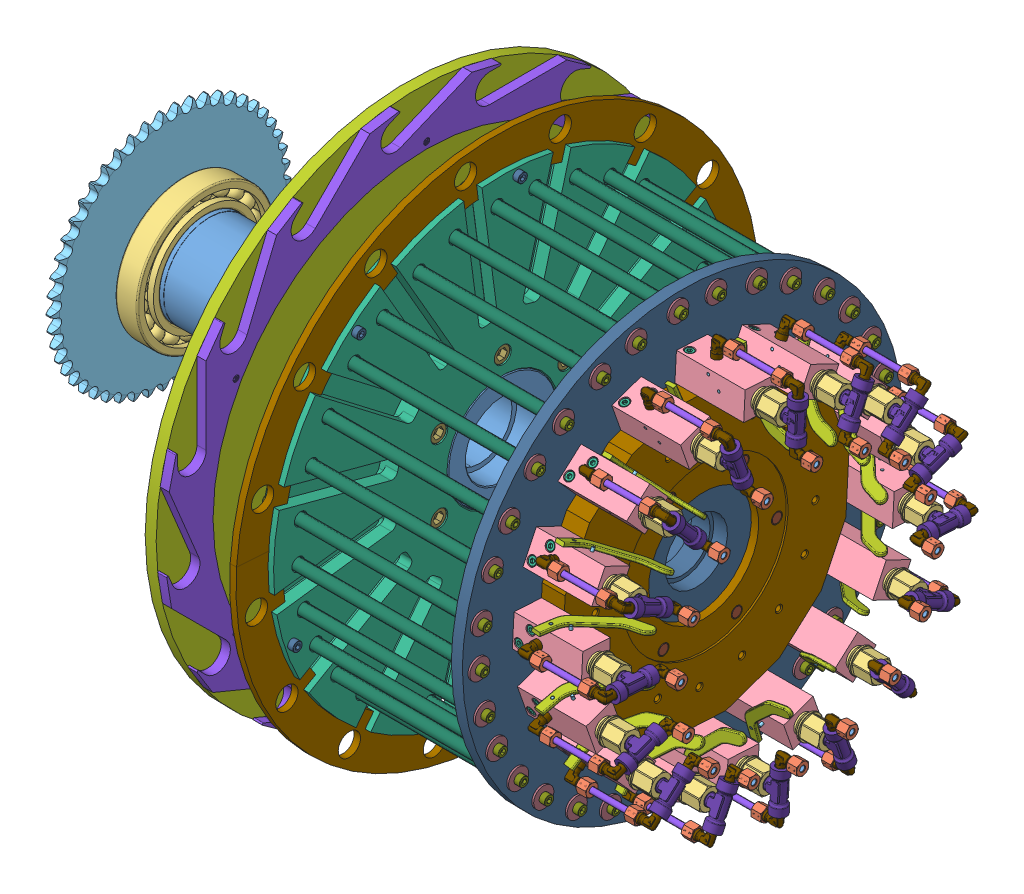
SolidWorks assembly assieme parte rotante, configuration Default. Lengths in mm.
Overall size (749.63 778.63 778.63).
555 component instances, 28 part files, 76 mates.
Components (placement in the parent):
- albero rotazione piatti-1: albero rotazione piatti [Default] at (60.413 18.3637 415) size (415 200 200)
- c-type retaining ring_external_ks-1: c-type retaining ring_external_ks [KS 1336 E - 100] at (-146.4567 18.3637 415) x (0 0 -1) z (1 0 0) size (107.55 112.98 3)
- SKF - 6020 - 20,DE,NC,20_68-1: SKF - 6020 - 20,DE,NC,20_68 [SKF - 6020 - 20,DE,NC,20_68] at (-131.4567 18.3637 415) x (1 0 0) z (0 -0.434476 -0.900684) size (24 150 150)
- calettatore d95-1: calettatore d95 [Default] at (-173.8867 18.3637 415) size (39.5 135 135)
- Chain wheel ISO - 50Z 10A-1-1: Chain wheel ISO - 50Z 10A-1 [Chain wheel ISO - 50Z 10A-1 --50SB120H25L95.0N] at (-164.8867 18.3637 415) size (29.89 262.06 262.51)
- Disco supporto montaggio e Colonne-1: Disco supporto montaggio e Colonne [Default] at (204.0433 18.3637 415) x (0 -0.866025 -0.5) z (1 0 0) size (499.6 499.6 29)
- SKF - 6020 - 20,DE,NC,20_68-2: SKF - 6020 - 20,DE,NC,20_68 [SKF - 6020 - 20,DE,NC,20_68] at (62.0433 18.3637 415) x (1 0 0) z (0 -0.432628 -0.901573) size (24 150 150)
- piatto rotante porta tappi-1: piatto rotante porta tappi [Default] at (99.0433 18.3637 415) x (0 0 -1) z (1 0 0) size (570 570 20.57)
- disco trasportatore tappi 31-1: disco trasportatore tappi 31 [Default] at (111.0433 18.3637 415) x (0 0.5 -0.866025) z (1 0 0) size (570 570 10.42)
- Distributore Rotante-1: Distributore Rotante [Default] at (425.0433 18.3637 415) x (0 -0.055301 -0.99847) z (1 0 0) size (310 310 25.54)
- disco trascinato porta distributore vuoto-1: disco trascinato porta distributore vuoto [Default] at (400.0433 18.3637 415) x (0 0.055301 0.99847) z (-1 0 0) size (480 480 50)
- m12 35mm-1: m12 35mm [ISO 4762 M12 x 35 - 35N] at (376.0433 -53.0243 378.8925) x (1 0 0) z (0 -0.5 0.866025) size (47 18 18)
- m12 90mm-3: m12 90mm [ISO 4762 M12 x 90 - 90N] at (203.0433 -21.6363 345.718) x (-1 0 0) z (0 -0.5 0.866025) size (102 18 18)
- rondella M10-1: rondella M10 [Washer ISO 7094 - 6] at (99.0433 -101.6363 207.1539) x (1 0 0) z (0 -1 0) size (2 22 22)
- M6 20mm-1: M6 20mm [ISO 4762 M6 x 20 - 20N] at (91.0433 -101.6363 207.1539) x (1 0 0) z (0 0.5 0.866025) size (26 10 10)
- m12 35mm-2: m12 35mm [ISO 4762 M12 x 35 - 35N] at (376.0433 13.9397 335.1224) x (1 0 0) z (0 -1 0) size (47 18 18)
- m12 35mm-3: m12 35mm [ISO 4762 M12 x 35 - 35N] at (376.0433 85.3277 371.2299) x (1 0 0) z (0 -0.5 -0.866025) size (47 18 18)
- m12 35mm-4: m12 35mm [ISO 4762 M12 x 35 - 35N] at (376.0433 89.7517 451.1075) x (1 0 0) z (0 0.5 -0.866025) size (47 18 18)
- m12 35mm-5: m12 35mm [ISO 4762 M12 x 35 - 35N] at (376.0433 22.7877 494.8776) x (1 0 0) z (0 1 0) size (47 18 18)
- m12 35mm-6: m12 35mm [ISO 4762 M12 x 35 - 35N] at (376.0433 -48.6003 458.7701) x (1 0 0) z (0 0.5 0.866025) size (47 18 18)
- rondella M10-2: rondella M10 [Washer ISO 7094 - 6] at (99.0433 138.3637 207.1539) x (1 0 0) z (0 -0.5 -0.866025) size (2 22 22)
- rondella M10-3: rondella M10 [Washer ISO 7094 - 6] at (99.0433 258.3637 415) x (1 0 0) z (0 0.5 -0.866025) size (2 22 22)
- rondella M10-4: rondella M10 [Washer ISO 7094 - 6] at (99.0433 138.3637 622.8461) x (1 0 0) z (0 1 0) size (2 22 22)
- rondella M10-5: rondella M10 [Washer ISO 7094 - 6] at (99.0433 -101.6363 622.8461) x (1 0 0) z (0 0.5 0.866025) size (2 22 22)
- rondella M10-6: rondella M10 [Washer ISO 7094 - 6] at (99.0433 -221.6363 415) x (1 0 0) z (0 -0.5 0.866025) size (2 22 22)
- M6 20mm-2: M6 20mm [ISO 4762 M6 x 20 - 20N] at (91.0433 138.3637 207.1539) x (1 0 0) z (0 -0.5 0.866025) size (26 10 10)
- M6 20mm-3: M6 20mm [ISO 4762 M6 x 20 - 20N] at (91.0433 258.3637 415) x (1 0 0) z (0 -1 0) size (26 10 10)
- M6 20mm-4: M6 20mm [ISO 4762 M6 x 20 - 20N] at (91.0433 138.3637 622.8461) x (1 0 0) z (0 -0.5 -0.866025) size (26 10 10)
- M6 20mm-5: M6 20mm [ISO 4762 M6 x 20 - 20N] at (91.0433 -101.6363 622.8461) x (1 0 0) z (0 0.5 -0.866025) size (26 10 10)
- M6 20mm-6: M6 20mm [ISO 4762 M6 x 20 - 20N] at (91.0433 -221.6363 415) x (1 0 0) z (0 1 0) size (26 10 10)
- m12 90mm-4: m12 90mm [ISO 4762 M12 x 90 - 90N] at (203.0433 58.3637 345.718) x (-1 0 0) z (0 -1 0) size (102 18 18)
- m12 90mm-5: m12 90mm [ISO 4762 M12 x 90 - 90N] at (203.0433 98.3637 415) x (-1 0 0) z (0 -0.5 -0.866025) size (102 18 18)
- m12 90mm-6: m12 90mm [ISO 4762 M12 x 90 - 90N] at (203.0433 58.3637 484.282) x (-1 0 0) z (0 0.5 -0.866025) size (102 18 18)
- m12 90mm-7: m12 90mm [ISO 4762 M12 x 90 - 90N] at (203.0433 -21.6363 484.282) x (-1 0 0) z (0 1 0) size (102 18 18)
- m12 90mm-8: m12 90mm [ISO 4762 M12 x 90 - 90N] at (203.0433 -61.6363 415) x (-1 0 0) z (0 0.5 0.866025) size (102 18 18)
- asta scorrimento carello-1: asta scorrimento carello [Default] at (287.5433 70.1437 197.9013) x (0 0 -1) z (1 0 0) size (12 12 225)
- rondella M10-7: rondella M10 [Washer ISO 7094 - 6] at (175.0433 70.1437 197.9013) x (1 0 0) z (0 -1 0) size (2 22 22)
- M6 16mm-1: M6 16mm [ISO 4762 M6 x 16 - 16N] at (167.0433 70.1437 197.9013) size (22 10 10)
- M6 16mm-2: M6 16mm [ISO 4762 M6 x 16 - 16N] at (408.0433 70.1437 197.9013) x (-1 0 0) z (0 0 -1) size (22 10 10)
- rondella M10-26: rondella M10 [Washer ISO 7094 - 6] at (400.0433 70.1437 197.9013) x (-1 0 0) z (0 1 0) size (2 22 22)
- rondella M10-42: rondella M10 [Washer ISO 7094 - 6] at (175.0433 24.5373 191.8971) x (1 0 0) z (0 -0.965926 -0.258819) size (2 22 22)
- M6 16mm-3: M6 16mm [ISO 4762 M6 x 16 - 16N] at (167.0433 24.5373 191.8971) x (1 0 0) z (0 0.258819 -0.965926) size (22 10 10)
- asta scorrimento carello-2: asta scorrimento carello [Default] at (287.5433 24.5373 191.8971) x (0 0.258819 -0.965926) z (-1 0 0) size (12 12 225)
- rondella M10-58: rondella M10 [Washer ISO 7094 - 6] at (400.0433 24.5373 191.8971) x (-1 0 0) z (0 0.965926 0.258819) size (2 22 22)
- M6 16mm-4: M6 16mm [ISO 4762 M6 x 16 - 16N] at (408.0433 24.5373 191.8971) x (-1 0 0) z (0 -0.258819 0.965926) size (22 10 10)
- AssiemeValvola-1: AssiemeValvola [Default] at (515.3257 74.6348 254.5832) x (0 -0.331007 0.943628) z (0 0.943628 0.331007) size (90.26 138.63 38)
  - RaccordoT-1: RaccordoT [Default] at origin size (43 29.75 16.5)
  - Raccordo a L-1: Raccordo a L [Default] at (-30 0 0) x (0 -1 0) z (0 0 -1) size (28.34 25.51 14.01)
    - 1809_06_10_01-1: 1809_06_10_01 [Default] at origin size (22.49 23 10)
    - 1809_06_10_02-1: 1809_06_10_02 [Default] at origin size (6.5 8.5 8.5)
    - 1809_06_10_03-1: 1809_06_10_03 [Default] at origin size (11.02 15.01 14.01)
  - Raccordo a L-2: Raccordo a L [Default] at (30 0 0) x (0 1 0) z (0 0 -1) size (28.34 25.51 14.01)
    - 1809_06_10_01-1: 1809_06_10_01 [Default] at origin size (22.49 23 10)
    - 1809_06_10_02-1: 1809_06_10_02 [Default] at origin size (6.5 8.5 8.5)
    - 1809_06_10_03-1: 1809_06_10_03 [Default] at origin size (11.02 15.01 14.01)
  - TappoChiusura-1: TappoChiusura [Default] at (0 -32 0) x (0 -1 0) z (0 0 1) size (38.28 26.74 26.74)
  - CorpoValvola-1: CorpoValvola [Default] at (-15 -115.2824 0) size (30 75 34)
  - Raccordo a L-3: Raccordo a L [Default] at (-30 -88.2824 0) x (0 1 0) z (0 0 1) size (28.34 25.51 14.01)
    - 1809_06_10_01-1: 1809_06_10_01 [Default] at origin size (22.49 23 10)
    - 1809_06_10_02-1: 1809_06_10_02 [Default] at origin size (6.5 8.5 8.5)
    - 1809_06_10_03-1: 1809_06_10_03 [Default] at origin size (11.02 15.01 14.01)
  - Spina_3x38-1: Spina_3x38 [Default] at (0 -68.2824 -21) x (-1 0 0) z (0 0 1) size (3 3 38)
  - Spina_3x38-2: Spina_3x38 [Default] at (-10 -80.2824 -21) x (0.996193 0.087174 0) z (0 0 1) size (3 3 38)
  - M5 40mm-3: M5 40mm [ISO 4762 M5 x 40 - 40N] at (-14.6 -108.7824 9) size (45 8.5 8.5)
  - M5 40mm-2: M5 40mm [ISO 4762 M5 x 40 - 40N] at (-14.6 -96.7824 -9) size (45 8.5 8.5)
  - LevaValvola-1: LevaValvola [Default] at (-24.507 -86.571 -17) x (0.996193 0.087174 0) z (0 0 1) size (77.55 60.2 4)
  - Tubo-1: Tubo [Default] at (-30 -15.9665 0) x (1 0 0) z (0 -1 0) size (6 6 56.4)
- M6 16mm-5: M6 16mm [ISO 4762 M6 x 16 - 16N] at (167.0433 -16.8778 194.6116) x (1 0 0) z (0 0.382683 0.92388) size (22 10 10)
- M6 16mm-6: M6 16mm [ISO 4762 M6 x 16 - 16N] at (167.0433 -98.5342 224.874) x (1 0 0) z (0 0.707107 0.707107) size (22 10 10)
- M6 16mm-7: M6 16mm [ISO 4762 M6 x 16 - 16N] at (167.0433 -162.3939 284.0814) x (1 0 0) z (0 0.92388 0.382683) size (22 10 10)
- M6 16mm-8: M6 16mm [ISO 4762 M6 x 16 - 16N] at (167.0433 -198.735 363.22) x (1 0 0) z (0 1 0) size (22 10 10)
- M6 16mm-9: M6 16mm [ISO 4762 M6 x 16 - 16N] at (167.0433 -202.0247 450.2415) x (1 0 0) z (0 0.92388 -0.382683) size (22 10 10)
- M6 16mm-10: M6 16mm [ISO 4762 M6 x 16 - 16N] at (167.0433 -171.7623 531.8979) x (1 0 0) z (0 0.707107 -0.707107) size (22 10 10)
- M6 16mm-11: M6 16mm [ISO 4762 M6 x 16 - 16N] at (167.0433 -112.5549 595.7576) x (1 0 0) z (0 0.382683 -0.92388) size (22 10 10)
- M6 16mm-12: M6 16mm [ISO 4762 M6 x 16 - 16N] at (167.0433 -33.4163 632.0987) x (1 0 0) z (0 0 -1) size (22 10 10)
- M6 16mm-13: M6 16mm [ISO 4762 M6 x 16 - 16N] at (167.0433 53.6052 635.3884) x (1 0 0) z (0 -0.382683 -0.92388) size (22 10 10)
- M6 16mm-14: M6 16mm [ISO 4762 M6 x 16 - 16N] at (167.0433 135.2616 605.126) x (1 0 0) z (0 -0.707107 -0.707107) size (22 10 10)
- M6 16mm-15: M6 16mm [ISO 4762 M6 x 16 - 16N] at (167.0433 199.1213 545.9186) x (1 0 0) z (0 -0.92388 -0.382683) size (22 10 10)
- M6 16mm-16: M6 16mm [ISO 4762 M6 x 16 - 16N] at (167.0433 235.4624 466.78) x (1 0 0) z (0 -1 0) size (22 10 10)
- M6 16mm-17: M6 16mm [ISO 4762 M6 x 16 - 16N] at (167.0433 238.7521 379.7585) x (1 0 0) z (0 -0.92388 0.382683) size (22 10 10)
- M6 16mm-18: M6 16mm [ISO 4762 M6 x 16 - 16N] at (167.0433 208.4897 298.1021) x (1 0 0) z (0 -0.707107 0.707107) size (22 10 10)
- M6 16mm-19: M6 16mm [ISO 4762 M6 x 16 - 16N] at (167.0433 149.2823 234.2424) x (1 0 0) z (0 -0.382683 0.92388) size (22 10 10)
- rondella M10-11: rondella M10 [Washer ISO 7094 - 6] at (175.0433 -16.8778 194.6116) x (1 0 0) z (0 -0.92388 0.382683) size (2 22 22)
- rondella M10-12: rondella M10 [Washer ISO 7094 - 6] at (175.0433 -98.5342 224.874) x (1 0 0) z (0 -0.707107 0.707107) size (2 22 22)
- rondella M10-13: rondella M10 [Washer ISO 7094 - 6] at (175.0433 -162.3939 284.0814) x (1 0 0) z (0 -0.382683 0.92388) size (2 22 22)
- rondella M10-14: rondella M10 [Washer ISO 7094 - 6] at (175.0433 -198.735 363.22) size (2 22 22)
- rondella M10-15: rondella M10 [Washer ISO 7094 - 6] at (175.0433 -202.0247 450.2415) x (1 0 0) z (0 0.382683 0.92388) size (2 22 22)
- rondella M10-16: rondella M10 [Washer ISO 7094 - 6] at (175.0433 -171.7623 531.8979) x (1 0 0) z (0 0.707107 0.707107) size (2 22 22)
- rondella M10-17: rondella M10 [Washer ISO 7094 - 6] at (175.0433 -112.5549 595.7576) x (1 0 0) z (0 0.92388 0.382683) size (2 22 22)
- rondella M10-18: rondella M10 [Washer ISO 7094 - 6] at (175.0433 -33.4163 632.0987) x (1 0 0) z (0 1 0) size (2 22 22)
- rondella M10-19: rondella M10 [Washer ISO 7094 - 6] at (175.0433 53.6052 635.3884) x (1 0 0) z (0 0.92388 -0.382683) size (2 22 22)
- rondella M10-20: rondella M10 [Washer ISO 7094 - 6] at (175.0433 135.2616 605.126) x (1 0 0) z (0 0.707107 -0.707107) size (2 22 22)
- rondella M10-21: rondella M10 [Washer ISO 7094 - 6] at (175.0433 199.1213 545.9186) x (1 0 0) z (0 0.382683 -0.92388) size (2 22 22)
- rondella M10-22: rondella M10 [Washer ISO 7094 - 6] at (175.0433 235.4624 466.78) x (1 0 0) z (0 0 -1) size (2 22 22)
- rondella M10-23: rondella M10 [Washer ISO 7094 - 6] at (175.0433 238.7521 379.7585) x (1 0 0) z (0 -0.382683 -0.92388) size (2 22 22)
- rondella M10-24: rondella M10 [Washer ISO 7094 - 6] at (175.0433 208.4897 298.1021) x (1 0 0) z (0 -0.707107 -0.707107) size (2 22 22)
- rondella M10-25: rondella M10 [Washer ISO 7094 - 6] at (175.0433 149.2823 234.2424) x (1 0 0) z (0 -0.92388 -0.382683) size (2 22 22)
- asta scorrimento carello-3: asta scorrimento carello [Default] at (287.5433 -16.8778 194.6116) x (0 -0.382683 -0.92388) z (1 0 0) size (12 12 225)
- asta scorrimento carello-4: asta scorrimento carello [Default] at (287.5433 -98.5342 224.874) x (0 -0.707107 -0.707107) z (1 0 0) size (12 12 225)
- asta scorrimento carello-5: asta scorrimento carello [Default] at (287.5433 -162.3939 284.0814) x (0 -0.92388 -0.382683) z (1 0 0) size (12 12 225)
- asta scorrimento carello-6: asta scorrimento carello [Default] at (287.5433 -198.735 363.22) x (0 -1 0) z (1 0 0) size (12 12 225)
- asta scorrimento carello-7: asta scorrimento carello [Default] at (287.5433 -202.0247 450.2415) x (0 -0.92388 0.382683) z (1 0 0) size (12 12 225)
- asta scorrimento carello-8: asta scorrimento carello [Default] at (287.5433 -171.7623 531.8979) x (0 -0.707107 0.707107) z (1 0 0) size (12 12 225)
- asta scorrimento carello-9: asta scorrimento carello [Default] at (287.5433 -112.5549 595.7576) x (0 -0.382683 0.92388) z (1 0 0) size (12 12 225)
- asta scorrimento carello-10: asta scorrimento carello [Default] at (287.5433 -33.4163 632.0987) x (0 0 1) z (1 0 0) size (12 12 225)
- asta scorrimento carello-11: asta scorrimento carello [Default] at (287.5433 53.6052 635.3884) x (0 0.382683 0.92388) z (1 0 0) size (12 12 225)
- asta scorrimento carello-12: asta scorrimento carello [Default] at (287.5433 135.2616 605.126) x (0 0.707107 0.707107) z (1 0 0) size (12 12 225)
- asta scorrimento carello-13: asta scorrimento carello [Default] at (287.5433 199.1213 545.9186) x (0 0.92388 0.382683) z (1 0 0) size (12 12 225)
- asta scorrimento carello-14: asta scorrimento carello [Default] at (287.5433 235.4624 466.78) x (0 1 0) z (1 0 0) size (12 12 225)
- asta scorrimento carello-15: asta scorrimento carello [Default] at (287.5433 238.7521 379.7585) x (0 0.92388 -0.382683) z (1 0 0) size (12 12 225)
- asta scorrimento carello-16: asta scorrimento carello [Default] at (287.5433 208.4897 298.1021) x (0 0.707107 -0.707107) z (1 0 0) size (12 12 225)
- asta scorrimento carello-17: asta scorrimento carello [Default] at (287.5433 149.2823 234.2424) x (0 0.382683 -0.92388) z (1 0 0) size (12 12 225)
- M6 16mm-20: M6 16mm [ISO 4762 M6 x 16 - 16N] at (408.0433 -16.8778 194.6116) x (-1 0 0) z (0 -0.382683 -0.92388) size (22 10 10)
- M6 16mm-21: M6 16mm [ISO 4762 M6 x 16 - 16N] at (408.0433 -98.5342 224.874) x (-1 0 0) z (0 -0.707107 -0.707107) size (22 10 10)
- M6 16mm-22: M6 16mm [ISO 4762 M6 x 16 - 16N] at (408.0433 -162.3939 284.0814) x (-1 0 0) z (0 -0.92388 -0.382683) size (22 10 10)
- M6 16mm-23: M6 16mm [ISO 4762 M6 x 16 - 16N] at (408.0433 -198.735 363.22) x (-1 0 0) z (0 -1 0) size (22 10 10)
- M6 16mm-24: M6 16mm [ISO 4762 M6 x 16 - 16N] at (408.0433 -202.0247 450.2415) x (-1 0 0) z (0 -0.92388 0.382683) size (22 10 10)
- M6 16mm-25: M6 16mm [ISO 4762 M6 x 16 - 16N] at (408.0433 -171.7623 531.8979) x (-1 0 0) z (0 -0.707107 0.707107) size (22 10 10)
- M6 16mm-26: M6 16mm [ISO 4762 M6 x 16 - 16N] at (408.0433 -112.5549 595.7576) x (-1 0 0) z (0 -0.382683 0.92388) size (22 10 10)
- M6 16mm-27: M6 16mm [ISO 4762 M6 x 16 - 16N] at (408.0433 -33.4163 632.0987) x (-1 0 0) z (0 0 1) size (22 10 10)
- M6 16mm-28: M6 16mm [ISO 4762 M6 x 16 - 16N] at (408.0433 53.6052 635.3884) x (-1 0 0) z (0 0.382683 0.92388) size (22 10 10)
- M6 16mm-29: M6 16mm [ISO 4762 M6 x 16 - 16N] at (408.0433 135.2616 605.126) x (-1 0 0) z (0 0.707107 0.707107) size (22 10 10)
- M6 16mm-30: M6 16mm [ISO 4762 M6 x 16 - 16N] at (408.0433 199.1213 545.9186) x (-1 0 0) z (0 0.92388 0.382683) size (22 10 10)
- M6 16mm-31: M6 16mm [ISO 4762 M6 x 16 - 16N] at (408.0433 235.4624 466.78) x (-1 0 0) z (0 1 0) size (22 10 10)
- M6 16mm-32: M6 16mm [ISO 4762 M6 x 16 - 16N] at (408.0433 238.7521 379.7585) x (-1 0 0) z (0 0.92388 -0.382683) size (22 10 10)
- M6 16mm-33: M6 16mm [ISO 4762 M6 x 16 - 16N] at (408.0433 208.4897 298.1021) x (-1 0 0) z (0 0.707107 -0.707107) size (22 10 10)
- M6 16mm-34: M6 16mm [ISO 4762 M6 x 16 - 16N] at (408.0433 149.2823 234.2424) x (-1 0 0) z (0 0.382683 -0.92388) size (22 10 10)
- rondella M10-27: rondella M10 [Washer ISO 7094 - 6] at (400.0433 -16.8778 194.6116) x (-1 0 0) z (0 0.92388 -0.382683) size (2 22 22)
- rondella M10-28: rondella M10 [Washer ISO 7094 - 6] at (400.0433 -98.5342 224.874) x (-1 0 0) z (0 0.707107 -0.707107) size (2 22 22)
- rondella M10-29: rondella M10 [Washer ISO 7094 - 6] at (400.0433 -162.3939 284.0814) x (-1 0 0) z (0 0.382683 -0.92388) size (2 22 22)
- rondella M10-30: rondella M10 [Washer ISO 7094 - 6] at (400.0433 -198.735 363.22) x (-1 0 0) z (0 0 -1) size (2 22 22)
- rondella M10-31: rondella M10 [Washer ISO 7094 - 6] at (400.0433 -202.0247 450.2415) x (-1 0 0) z (0 -0.382683 -0.92388) size (2 22 22)
- rondella M10-32: rondella M10 [Washer ISO 7094 - 6] at (400.0433 -171.7623 531.8979) x (-1 0 0) z (0 -0.707107 -0.707107) size (2 22 22)
- rondella M10-33: rondella M10 [Washer ISO 7094 - 6] at (400.0433 -112.5549 595.7576) x (-1 0 0) z (0 -0.92388 -0.382683) size (2 22 22)
- rondella M10-34: rondella M10 [Washer ISO 7094 - 6] at (400.0433 -33.4163 632.0987) x (-1 0 0) z (0 -1 0) size (2 22 22)
- rondella M10-35: rondella M10 [Washer ISO 7094 - 6] at (400.0433 53.6052 635.3884) x (-1 0 0) z (0 -0.92388 0.382683) size (2 22 22)
- rondella M10-36: rondella M10 [Washer ISO 7094 - 6] at (400.0433 135.2616 605.126) x (-1 0 0) z (0 -0.707107 0.707107) size (2 22 22)
- rondella M10-37: rondella M10 [Washer ISO 7094 - 6] at (400.0433 199.1213 545.9186) x (-1 0 0) z (0 -0.382683 0.92388) size (2 22 22)
- rondella M10-38: rondella M10 [Washer ISO 7094 - 6] at (400.0433 235.4624 466.78) x (-1 0 0) z (0 0 1) size (2 22 22)
- rondella M10-39: rondella M10 [Washer ISO 7094 - 6] at (400.0433 238.7521 379.7585) x (-1 0 0) z (0 0.382683 0.92388) size (2 22 22)
- rondella M10-40: rondella M10 [Washer ISO 7094 - 6] at (400.0433 208.4897 298.1021) x (-1 0 0) z (0 0.707107 0.707107) size (2 22 22)
- rondella M10-41: rondella M10 [Washer ISO 7094 - 6] at (400.0433 149.2823 234.2424) x (-1 0 0) z (0 0.92388 0.382683) size (2 22 22)
- rondella M10-43: rondella M10 [Washer ISO 7094 - 6] at (175.0433 -61.3104 206.5173) x (1 0 0) z (0 -0.991445 0.130526) size (2 22 22)
- rondella M10-44: rondella M10 [Washer ISO 7094 - 6] at (175.0433 -135.0285 252.8771) x (1 0 0) z (0 -0.866025 0.5) size (2 22 22)
- rondella M10-45: rondella M10 [Washer ISO 7094 - 6] at (175.0433 -185.3939 323.9186) x (1 0 0) z (0 -0.608761 0.793353) size (2 22 22)
- rondella M10-46: rondella M10 [Washer ISO 7094 - 6] at (175.0433 -204.7392 408.8264) x (1 0 0) z (0 -0.258819 0.965926) size (2 22 22)
- rondella M10-47: rondella M10 [Washer ISO 7094 - 6] at (175.0433 -190.119 494.6741) x (1 0 0) z (0 0.130526 0.991445) size (2 22 22)
- rondella M10-48: rondella M10 [Washer ISO 7094 - 6] at (175.0433 -143.7592 568.3922) x (1 0 0) z (0 0.5 0.866025) size (2 22 22)
- rondella M10-49: rondella M10 [Washer ISO 7094 - 6] at (175.0433 -72.7177 618.7576) x (1 0 0) z (0 0.793353 0.608761) size (2 22 22)
- rondella M10-50: rondella M10 [Washer ISO 7094 - 6] at (175.0433 12.1901 638.1029) x (1 0 0) z (0 0.965926 0.258819) size (2 22 22)
- rondella M10-51: rondella M10 [Washer ISO 7094 - 6] at (175.0433 98.0378 623.4827) x (1 0 0) z (0 0.991445 -0.130526) size (2 22 22)
- rondella M10-52: rondella M10 [Washer ISO 7094 - 6] at (175.0433 171.7559 577.1229) x (1 0 0) z (0 0.866025 -0.5) size (2 22 22)
- rondella M10-53: rondella M10 [Washer ISO 7094 - 6] at (175.0433 222.1213 506.0814) x (1 0 0) z (0 0.608761 -0.793353) size (2 22 22)
- rondella M10-54: rondella M10 [Washer ISO 7094 - 6] at (175.0433 241.4666 421.1736) x (1 0 0) z (0 0.258819 -0.965926) size (2 22 22)
- rondella M10-55: rondella M10 [Washer ISO 7094 - 6] at (175.0433 226.8464 335.3259) x (1 0 0) z (0 -0.130526 -0.991445) size (2 22 22)
- rondella M10-56: rondella M10 [Washer ISO 7094 - 6] at (175.0433 180.4866 261.6078) x (1 0 0) z (0 -0.5 -0.866025) size (2 22 22)
- rondella M10-57: rondella M10 [Washer ISO 7094 - 6] at (175.0433 109.4451 211.2424) x (1 0 0) z (0 -0.793353 -0.608761) size (2 22 22)
- M6 16mm-35: M6 16mm [ISO 4762 M6 x 16 - 16N] at (167.0433 -61.3104 206.5173) x (1 0 0) z (0 -0.130526 -0.991445) size (22 10 10)
- M6 16mm-36: M6 16mm [ISO 4762 M6 x 16 - 16N] at (167.0433 -135.0285 252.8771) x (1 0 0) z (0 -0.5 -0.866025) size (22 10 10)
- M6 16mm-37: M6 16mm [ISO 4762 M6 x 16 - 16N] at (167.0433 -185.3939 323.9186) x (1 0 0) z (0 -0.793353 -0.608761) size (22 10 10)
- M6 16mm-38: M6 16mm [ISO 4762 M6 x 16 - 16N] at (167.0433 -204.7392 408.8264) x (1 0 0) z (0 -0.965926 -0.258819) size (22 10 10)
- M6 16mm-39: M6 16mm [ISO 4762 M6 x 16 - 16N] at (167.0433 -190.119 494.6741) x (1 0 0) z (0 -0.991445 0.130526) size (22 10 10)
- M6 16mm-40: M6 16mm [ISO 4762 M6 x 16 - 16N] at (167.0433 -143.7592 568.3922) x (1 0 0) z (0 -0.866025 0.5) size (22 10 10)
- M6 16mm-41: M6 16mm [ISO 4762 M6 x 16 - 16N] at (167.0433 -72.7177 618.7576) x (1 0 0) z (0 -0.608761 0.793353) size (22 10 10)
- M6 16mm-42: M6 16mm [ISO 4762 M6 x 16 - 16N] at (167.0433 12.1901 638.1029) x (1 0 0) z (0 -0.258819 0.965926) size (22 10 10)
- M6 16mm-43: M6 16mm [ISO 4762 M6 x 16 - 16N] at (167.0433 98.0378 623.4827) x (1 0 0) z (0 0.130526 0.991445) size (22 10 10)
- M6 16mm-44: M6 16mm [ISO 4762 M6 x 16 - 16N] at (167.0433 171.7559 577.1229) x (1 0 0) z (0 0.5 0.866025) size (22 10 10)
- M6 16mm-45: M6 16mm [ISO 4762 M6 x 16 - 16N] at (167.0433 222.1213 506.0814) x (1 0 0) z (0 0.793353 0.608761) size (22 10 10)
- M6 16mm-46: M6 16mm [ISO 4762 M6 x 16 - 16N] at (167.0433 241.4666 421.1736) x (1 0 0) z (0 0.965926 0.258819) size (22 10 10)
- M6 16mm-47: M6 16mm [ISO 4762 M6 x 16 - 16N] at (167.0433 226.8464 335.3259) x (1 0 0) z (0 0.991445 -0.130526) size (22 10 10)
- M6 16mm-48: M6 16mm [ISO 4762 M6 x 16 - 16N] at (167.0433 180.4866 261.6078) x (1 0 0) z (0 0.866025 -0.5) size (22 10 10)
- M6 16mm-49: M6 16mm [ISO 4762 M6 x 16 - 16N] at (167.0433 109.4451 211.2424) x (1 0 0) z (0 0.608761 -0.793353) size (22 10 10)
- asta scorrimento carello-18: asta scorrimento carello [Default] at (287.5433 -61.3104 206.5173) x (0 -0.130526 -0.991445) z (-1 0 0) size (12 12 225)
- asta scorrimento carello-19: asta scorrimento carello [Default] at (287.5433 -135.0285 252.8771) x (0 -0.5 -0.866025) z (-1 0 0) size (12 12 225)
- asta scorrimento carello-20: asta scorrimento carello [Default] at (287.5433 -185.3939 323.9186) x (0 -0.793353 -0.608761) z (-1 0 0) size (12 12 225)
- asta scorrimento carello-21: asta scorrimento carello [Default] at (287.5433 -204.7392 408.8264) x (0 -0.965926 -0.258819) z (-1 0 0) size (12 12 225)
- asta scorrimento carello-22: asta scorrimento carello [Default] at (287.5433 -190.119 494.6741) x (0 -0.991445 0.130526) z (-1 0 0) size (12 12 225)
- asta scorrimento carello-23: asta scorrimento carello [Default] at (287.5433 -143.7592 568.3922) x (0 -0.866025 0.5) z (-1 0 0) size (12 12 225)
- asta scorrimento carello-24: asta scorrimento carello [Default] at (287.5433 -72.7177 618.7576) x (0 -0.608761 0.793353) z (-1 0 0) size (12 12 225)
- asta scorrimento carello-25: asta scorrimento carello [Default] at (287.5433 12.1901 638.1029) x (0 -0.258819 0.965926) z (-1 0 0) size (12 12 225)
- asta scorrimento carello-26: asta scorrimento carello [Default] at (287.5433 98.0378 623.4827) x (0 0.130526 0.991445) z (-1 0 0) size (12 12 225)
- asta scorrimento carello-27: asta scorrimento carello [Default] at (287.5433 171.7559 577.1229) x (0 0.5 0.866025) z (-1 0 0) size (12 12 225)
- asta scorrimento carello-28: asta scorrimento carello [Default] at (287.5433 222.1213 506.0814) x (0 0.793353 0.608761) z (-1 0 0) size (12 12 225)
- asta scorrimento carello-29: asta scorrimento carello [Default] at (287.5433 241.4666 421.1736) x (0 0.965926 0.258819) z (-1 0 0) size (12 12 225)
- asta scorrimento carello-30: asta scorrimento carello [Default] at (287.5433 226.8464 335.3259) x (0 0.991445 -0.130526) z (-1 0 0) size (12 12 225)
- asta scorrimento carello-31: asta scorrimento carello [Default] at (287.5433 180.4866 261.6078) x (0 0.866025 -0.5) z (-1 0 0) size (12 12 225)
- asta scorrimento carello-32: asta scorrimento carello [Default] at (287.5433 109.4451 211.2424) x (0 0.608761 -0.793353) z (-1 0 0) size (12 12 225)
- rondella M10-59: rondella M10 [Washer ISO 7094 - 6] at (400.0433 -61.3104 206.5173) x (-1 0 0) z (0 0.991445 -0.130526) size (2 22 22)
- rondella M10-60: rondella M10 [Washer ISO 7094 - 6] at (400.0433 -135.0285 252.8771) x (-1 0 0) z (0 0.866025 -0.5) size (2 22 22)
- rondella M10-61: rondella M10 [Washer ISO 7094 - 6] at (400.0433 -185.3939 323.9186) x (-1 0 0) z (0 0.608761 -0.793353) size (2 22 22)
- rondella M10-62: rondella M10 [Washer ISO 7094 - 6] at (400.0433 -204.7392 408.8264) x (-1 0 0) z (0 0.258819 -0.965926) size (2 22 22)
- rondella M10-63: rondella M10 [Washer ISO 7094 - 6] at (400.0433 -190.119 494.6741) x (-1 0 0) z (0 -0.130526 -0.991445) size (2 22 22)
- rondella M10-64: rondella M10 [Washer ISO 7094 - 6] at (400.0433 -143.7592 568.3922) x (-1 0 0) z (0 -0.5 -0.866025) size (2 22 22)
- rondella M10-65: rondella M10 [Washer ISO 7094 - 6] at (400.0433 -72.7177 618.7576) x (-1 0 0) z (0 -0.793353 -0.608761) size (2 22 22)
- rondella M10-66: rondella M10 [Washer ISO 7094 - 6] at (400.0433 12.1901 638.1029) x (-1 0 0) z (0 -0.965926 -0.258819) size (2 22 22)
- rondella M10-67: rondella M10 [Washer ISO 7094 - 6] at (400.0433 98.0378 623.4827) x (-1 0 0) z (0 -0.991445 0.130526) size (2 22 22)
- rondella M10-68: rondella M10 [Washer ISO 7094 - 6] at (400.0433 171.7559 577.1229) x (-1 0 0) z (0 -0.866025 0.5) size (2 22 22)
- rondella M10-69: rondella M10 [Washer ISO 7094 - 6] at (400.0433 222.1213 506.0814) x (-1 0 0) z (0 -0.608761 0.793353) size (2 22 22)
- rondella M10-70: rondella M10 [Washer ISO 7094 - 6] at (400.0433 241.4666 421.1736) x (-1 0 0) z (0 -0.258819 0.965926) size (2 22 22)
- rondella M10-71: rondella M10 [Washer ISO 7094 - 6] at (400.0433 226.8464 335.3259) x (-1 0 0) z (0 0.130526 0.991445) size (2 22 22)
- rondella M10-72: rondella M10 [Washer ISO 7094 - 6] at (400.0433 180.4866 261.6078) x (-1 0 0) z (0 0.5 0.866025) size (2 22 22)
- rondella M10-73: rondella M10 [Washer ISO 7094 - 6] at (400.0433 109.4451 211.2424) x (-1 0 0) z (0 0.793353 0.608761) size (2 22 22)
- M6 16mm-50: M6 16mm [ISO 4762 M6 x 16 - 16N] at (408.0433 -61.3104 206.5173) x (-1 0 0) z (0 0.130526 0.991445) size (22 10 10)
- M6 16mm-51: M6 16mm [ISO 4762 M6 x 16 - 16N] at (408.0433 -135.0285 252.8771) x (-1 0 0) z (0 0.5 0.866025) size (22 10 10)
- M6 16mm-52: M6 16mm [ISO 4762 M6 x 16 - 16N] at (408.0433 -185.3939 323.9186) x (-1 0 0) z (0 0.793353 0.608761) size (22 10 10)
- M6 16mm-53: M6 16mm [ISO 4762 M6 x 16 - 16N] at (408.0433 -204.7392 408.8264) x (-1 0 0) z (0 0.965926 0.258819) size (22 10 10)
- M6 16mm-54: M6 16mm [ISO 4762 M6 x 16 - 16N] at (408.0433 -190.119 494.6741) x (-1 0 0) z (0 0.991445 -0.130526) size (22 10 10)
- M6 16mm-55: M6 16mm [ISO 4762 M6 x 16 - 16N] at (408.0433 -143.7592 568.3922) x (-1 0 0) z (0 0.866025 -0.5) size (22 10 10)
- M6 16mm-56: M6 16mm [ISO 4762 M6 x 16 - 16N] at (408.0433 -72.7177 618.7576) x (-1 0 0) z (0 0.608761 -0.793353) size (22 10 10)
- M6 16mm-57: M6 16mm [ISO 4762 M6 x 16 - 16N] at (408.0433 12.1901 638.1029) x (-1 0 0) z (0 0.258819 -0.965926) size (22 10 10)
- M6 16mm-58: M6 16mm [ISO 4762 M6 x 16 - 16N] at (408.0433 98.0378 623.4827) x (-1 0 0) z (0 -0.130526 -0.991445) size (22 10 10)
- M6 16mm-59: M6 16mm [ISO 4762 M6 x 16 - 16N] at (408.0433 171.7559 577.1229) x (-1 0 0) z (0 -0.5 -0.866025) size (22 10 10)
- M6 16mm-60: M6 16mm [ISO 4762 M6 x 16 - 16N] at (408.0433 222.1213 506.0814) x (-1 0 0) z (0 -0.793353 -0.608761) size (22 10 10)
- M6 16mm-61: M6 16mm [ISO 4762 M6 x 16 - 16N] at (408.0433 241.4666 421.1736) x (-1 0 0) z (0 -0.965926 -0.258819) size (22 10 10)
- M6 16mm-62: M6 16mm [ISO 4762 M6 x 16 - 16N] at (408.0433 226.8464 335.3259) x (-1 0 0) z (0 -0.991445 0.130526) size (22 10 10)
- M6 16mm-63: M6 16mm [ISO 4762 M6 x 16 - 16N] at (408.0433 180.4866 261.6078) x (-1 0 0) z (0 -0.866025 0.5) size (22 10 10)
- M6 16mm-64: M6 16mm [ISO 4762 M6 x 16 - 16N] at (408.0433 109.4451 211.2424) x (-1 0 0) z (0 -0.608761 0.793353) size (22 10 10)
- AssiemeValvola-2: AssiemeValvola [Default] at (515.3257 8.9626 245.2601) x (0 0.055301 0.99847) z (0 0.99847 -0.055301) size (90.26 138.63 38)
  - RaccordoT-1: RaccordoT [Default] at origin size (43 29.75 16.5)
  - Raccordo a L-1: Raccordo a L [Default] at (-30 0 0) x (0 -1 0) z (0 0 -1) size (28.34 25.51 14.01)
    - 1809_06_10_01-1: 1809_06_10_01 [Default] at origin size (22.49 23 10)
    - 1809_06_10_02-1: 1809_06_10_02 [Default] at origin size (6.5 8.5 8.5)
    - 1809_06_10_03-1: 1809_06_10_03 [Default] at origin size (11.02 15.01 14.01)
  - Raccordo a L-2: Raccordo a L [Default] at (30 0 0) x (0 1 0) z (0 0 -1) size (28.34 25.51 14.01)
    - 1809_06_10_01-1: 1809_06_10_01 [Default] at origin size (22.49 23 10)
    - 1809_06_10_02-1: 1809_06_10_02 [Default] at origin size (6.5 8.5 8.5)
    - 1809_06_10_03-1: 1809_06_10_03 [Default] at origin size (11.02 15.01 14.01)
  - TappoChiusura-1: TappoChiusura [Default] at (0 -32 0) x (0 -1 0) z (0 0 1) size (38.28 26.74 26.74)
  - CorpoValvola-1: CorpoValvola [Default] at (-15 -115.2824 0) size (30 75 34)
  - Raccordo a L-3: Raccordo a L [Default] at (-30 -88.2824 0) x (0 1 0) z (0 0 1) size (28.34 25.51 14.01)
    - 1809_06_10_01-1: 1809_06_10_01 [Default] at origin size (22.49 23 10)
    - 1809_06_10_02-1: 1809_06_10_02 [Default] at origin size (6.5 8.5 8.5)
    - 1809_06_10_03-1: 1809_06_10_03 [Default] at origin size (11.02 15.01 14.01)
  - Spina_3x38-1: Spina_3x38 [Default] at (0 -68.2824 -21) x (-1 0 0) z (0 0 1) size (3 3 38)
  - Spina_3x38-2: Spina_3x38 [Default] at (-10 -80.2824 -21) x (0.996193 0.087174 0) z (0 0 1) size (3 3 38)
  - M5 40mm-3: M5 40mm [ISO 4762 M5 x 40 - 40N] at (-14.6 -108.7824 9) size (45 8.5 8.5)
  - M5 40mm-2: M5 40mm [ISO 4762 M5 x 40 - 40N] at (-14.6 -96.7824 -9) size (45 8.5 8.5)
  - LevaValvola-1: LevaValvola [Default] at (-24.507 -86.571 -17) x (0.996193 0.087174 0) z (0 0 1) size (77.55 60.2 4)
  - Tubo-1: Tubo [Default] at (-30 -15.9665 0) x (1 0 0) z (0 -1 0) size (6 6 56.4)
- AssiemeValvola-3: AssiemeValvola [Default] at (515.3257 -55.2784 261.7785) x (0 0.433189 0.901303) z (0 0.901303 -0.433189) size (90.26 138.63 38)
  - RaccordoT-1: RaccordoT [Default] at origin size (43 29.75 16.5)
  - Raccordo a L-1: Raccordo a L [Default] at (-30 0 0) x (0 -1 0) z (0 0 -1) size (28.34 25.51 14.01)
    - 1809_06_10_01-1: 1809_06_10_01 [Default] at origin size (22.49 23 10)
    - 1809_06_10_02-1: 1809_06_10_02 [Default] at origin size (6.5 8.5 8.5)
    - 1809_06_10_03-1: 1809_06_10_03 [Default] at origin size (11.02 15.01 14.01)
  - Raccordo a L-2: Raccordo a L [Default] at (30 0 0) x (0 1 0) z (0 0 -1) size (28.34 25.51 14.01)
    - 1809_06_10_01-1: 1809_06_10_01 [Default] at origin size (22.49 23 10)
    - 1809_06_10_02-1: 1809_06_10_02 [Default] at origin size (6.5 8.5 8.5)
    - 1809_06_10_03-1: 1809_06_10_03 [Default] at origin size (11.02 15.01 14.01)
  - TappoChiusura-1: TappoChiusura [Default] at (0 -32 0) x (0 -1 0) z (0 0 1) size (38.28 26.74 26.74)
  - CorpoValvola-1: CorpoValvola [Default] at (-15 -115.2824 0) size (30 75 34)
  - Raccordo a L-3: Raccordo a L [Default] at (-30 -88.2824 0) x (0 1 0) z (0 0 1) size (28.34 25.51 14.01)
    - 1809_06_10_01-1: 1809_06_10_01 [Default] at origin size (22.49 23 10)
    - 1809_06_10_02-1: 1809_06_10_02 [Default] at origin size (6.5 8.5 8.5)
    - 1809_06_10_03-1: 1809_06_10_03 [Default] at origin size (11.02 15.01 14.01)
  - Spina_3x38-1: Spina_3x38 [Default] at (0 -68.2824 -21) x (-1 0 0) z (0 0 1) size (3 3 38)
  - Spina_3x38-2: Spina_3x38 [Default] at (-10 -80.2824 -21) x (0.996193 0.087174 0) z (0 0 1) size (3 3 38)
  - M5 40mm-3: M5 40mm [ISO 4762 M5 x 40 - 40N] at (-14.6 -108.7824 9) size (45 8.5 8.5)
  - M5 40mm-2: M5 40mm [ISO 4762 M5 x 40 - 40N] at (-14.6 -96.7824 -9) size (45 8.5 8.5)
  - LevaValvola-1: LevaValvola [Default] at (-24.507 -86.571 -17) x (0.996193 0.087174 0) z (0 0 1) size (77.55 60.2 4)
  - Tubo-1: Tubo [Default] at (-30 -15.9665 0) x (1 0 0) z (0 -1 0) size (6 6 56.4)
- AssiemeValvola-4: AssiemeValvola [Default] at (515.3257 -108.3081 301.6234) x (0 0.745128 0.666921) z (0 0.666921 -0.745128) size (90.26 138.63 38)
  - RaccordoT-1: RaccordoT [Default] at origin size (43 29.75 16.5)
  - Raccordo a L-1: Raccordo a L [Default] at (-30 0 0) x (0 -1 0) z (0 0 -1) size (28.34 25.51 14.01)
    - 1809_06_10_01-1: 1809_06_10_01 [Default] at origin size (22.49 23 10)
    - 1809_06_10_02-1: 1809_06_10_02 [Default] at origin size (6.5 8.5 8.5)
    - 1809_06_10_03-1: 1809_06_10_03 [Default] at origin size (11.02 15.01 14.01)
  - Raccordo a L-2: Raccordo a L [Default] at (30 0 0) x (0 1 0) z (0 0 -1) size (28.34 25.51 14.01)
    - 1809_06_10_01-1: 1809_06_10_01 [Default] at origin size (22.49 23 10)
    - 1809_06_10_02-1: 1809_06_10_02 [Default] at origin size (6.5 8.5 8.5)
    - 1809_06_10_03-1: 1809_06_10_03 [Default] at origin size (11.02 15.01 14.01)
  - TappoChiusura-1: TappoChiusura [Default] at (0 -32 0) x (0 -1 0) z (0 0 1) size (38.28 26.74 26.74)
  - CorpoValvola-1: CorpoValvola [Default] at (-15 -115.2824 0) size (30 75 34)
  - Raccordo a L-3: Raccordo a L [Default] at (-30 -88.2824 0) x (0 1 0) z (0 0 1) size (28.34 25.51 14.01)
    - 1809_06_10_01-1: 1809_06_10_01 [Default] at origin size (22.49 23 10)
    - 1809_06_10_02-1: 1809_06_10_02 [Default] at origin size (6.5 8.5 8.5)
    - 1809_06_10_03-1: 1809_06_10_03 [Default] at origin size (11.02 15.01 14.01)
  - Spina_3x38-1: Spina_3x38 [Default] at (0 -68.2824 -21) x (-1 0 0) z (0 0 1) size (3 3 38)
  - Spina_3x38-2: Spina_3x38 [Default] at (-10 -80.2824 -21) x (0.996193 0.087174 0) z (0 0 1) size (3 3 38)
  - M5 40mm-3: M5 40mm [ISO 4762 M5 x 40 - 40N] at (-14.6 -108.7824 9) size (45 8.5 8.5)
  - M5 40mm-2: M5 40mm [ISO 4762 M5 x 40 - 40N] at (-14.6 -96.7824 -9) size (45 8.5 8.5)
  - LevaValvola-1: LevaValvola [Default] at (-24.507 -86.571 -17) x (0.996193 0.087174 0) z (0 0 1) size (77.55 60.2 4)
  - Tubo-1: Tubo [Default] at (-30 -15.9665 0) x (1 0 0) z (0 -1 0) size (6 6 56.4)
- AssiemeValvola-5: AssiemeValvola [Default] at (515.3257 -142.0531 358.7289) x (0 0.943628 0.331007) z (0 0.331007 -0.943628) size (90.26 138.63 38)
  - RaccordoT-1: RaccordoT [Default] at origin size (43 29.75 16.5)
  - Raccordo a L-1: Raccordo a L [Default] at (-30 0 0) x (0 -1 0) z (0 0 -1) size (28.34 25.51 14.01)
    - 1809_06_10_01-1: 1809_06_10_01 [Default] at origin size (22.49 23 10)
    - 1809_06_10_02-1: 1809_06_10_02 [Default] at origin size (6.5 8.5 8.5)
    - 1809_06_10_03-1: 1809_06_10_03 [Default] at origin size (11.02 15.01 14.01)
  - Raccordo a L-2: Raccordo a L [Default] at (30 0 0) x (0 1 0) z (0 0 -1) size (28.34 25.51 14.01)
    - 1809_06_10_01-1: 1809_06_10_01 [Default] at origin size (22.49 23 10)
    - 1809_06_10_02-1: 1809_06_10_02 [Default] at origin size (6.5 8.5 8.5)
    - 1809_06_10_03-1: 1809_06_10_03 [Default] at origin size (11.02 15.01 14.01)
  - TappoChiusura-1: TappoChiusura [Default] at (0 -32 0) x (0 -1 0) z (0 0 1) size (38.28 26.74 26.74)
  - CorpoValvola-1: CorpoValvola [Default] at (-15 -115.2824 0) size (30 75 34)
  - Raccordo a L-3: Raccordo a L [Default] at (-30 -88.2824 0) x (0 1 0) z (0 0 1) size (28.34 25.51 14.01)
    - 1809_06_10_01-1: 1809_06_10_01 [Default] at origin size (22.49 23 10)
    - 1809_06_10_02-1: 1809_06_10_02 [Default] at origin size (6.5 8.5 8.5)
    - 1809_06_10_03-1: 1809_06_10_03 [Default] at origin size (11.02 15.01 14.01)
  - Spina_3x38-1: Spina_3x38 [Default] at (0 -68.2824 -21) x (-1 0 0) z (0 0 1) size (3 3 38)
  - Spina_3x38-2: Spina_3x38 [Default] at (-10 -80.2824 -21) x (0.996193 0.087174 0) z (0 0 1) size (3 3 38)
  - M5 40mm-3: M5 40mm [ISO 4762 M5 x 40 - 40N] at (-14.6 -108.7824 9) size (45 8.5 8.5)
  - M5 40mm-2: M5 40mm [ISO 4762 M5 x 40 - 40N] at (-14.6 -96.7824 -9) size (45 8.5 8.5)
  - LevaValvola-1: LevaValvola [Default] at (-24.507 -86.571 -17) x (0.996193 0.087174 0) z (0 0 1) size (77.55 60.2 4)
  - Tubo-1: Tubo [Default] at (-30 -15.9665 0) x (1 0 0) z (0 -1 0) size (6 6 56.4)
- AssiemeValvola-6: AssiemeValvola [Default] at (515.3257 -151.3762 424.4011) x (0 0.99847 -0.055301) z (0 -0.055301 -0.99847) size (90.26 138.63 38)
  - RaccordoT-1: RaccordoT [Default] at origin size (43 29.75 16.5)
  - Raccordo a L-1: Raccordo a L [Default] at (-30 0 0) x (0 -1 0) z (0 0 -1) size (28.34 25.51 14.01)
    - 1809_06_10_01-1: 1809_06_10_01 [Default] at origin size (22.49 23 10)
    - 1809_06_10_02-1: 1809_06_10_02 [Default] at origin size (6.5 8.5 8.5)
    - 1809_06_10_03-1: 1809_06_10_03 [Default] at origin size (11.02 15.01 14.01)
  - Raccordo a L-2: Raccordo a L [Default] at (30 0 0) x (0 1 0) z (0 0 -1) size (28.34 25.51 14.01)
    - 1809_06_10_01-1: 1809_06_10_01 [Default] at origin size (22.49 23 10)
    - 1809_06_10_02-1: 1809_06_10_02 [Default] at origin size (6.5 8.5 8.5)
    - 1809_06_10_03-1: 1809_06_10_03 [Default] at origin size (11.02 15.01 14.01)
  - TappoChiusura-1: TappoChiusura [Default] at (0 -32 0) x (0 -1 0) z (0 0 1) size (38.28 26.74 26.74)
  - CorpoValvola-1: CorpoValvola [Default] at (-15 -115.2824 0) size (30 75 34)
  - Raccordo a L-3: Raccordo a L [Default] at (-30 -88.2824 0) x (0 1 0) z (0 0 1) size (28.34 25.51 14.01)
    - 1809_06_10_01-1: 1809_06_10_01 [Default] at origin size (22.49 23 10)
    - 1809_06_10_02-1: 1809_06_10_02 [Default] at origin size (6.5 8.5 8.5)
    - 1809_06_10_03-1: 1809_06_10_03 [Default] at origin size (11.02 15.01 14.01)
  - Spina_3x38-1: Spina_3x38 [Default] at (0 -68.2824 -21) x (-1 0 0) z (0 0 1) size (3 3 38)
  - Spina_3x38-2: Spina_3x38 [Default] at (-10 -80.2824 -21) x (0.996193 0.087174 0) z (0 0 1) size (3 3 38)
  - M5 40mm-3: M5 40mm [ISO 4762 M5 x 40 - 40N] at (-14.6 -108.7824 9) size (45 8.5 8.5)
  - M5 40mm-2: M5 40mm [ISO 4762 M5 x 40 - 40N] at (-14.6 -96.7824 -9) size (45 8.5 8.5)
  - LevaValvola-1: LevaValvola [Default] at (-24.507 -86.571 -17) x (0.996193 0.087174 0) z (0 0 1) size (77.55 60.2 4)
  - Tubo-1: Tubo [Default] at (-30 -15.9665 0) x (1 0 0) z (0 -1 0) size (6 6 56.4)
